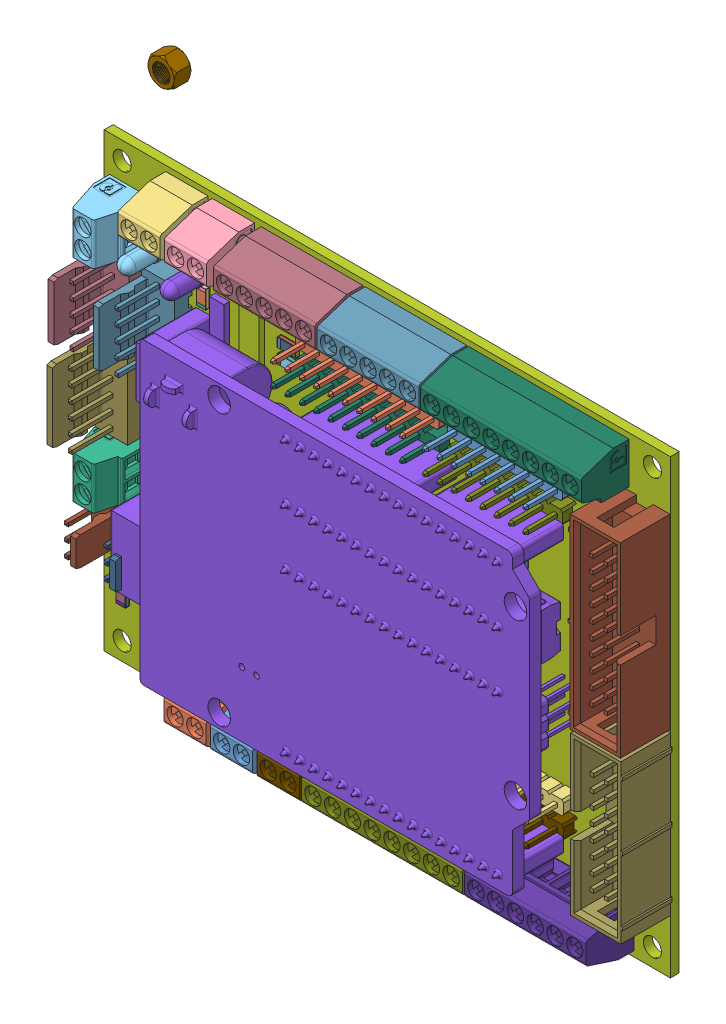
SolidWorks assembly Arduino Uno shield with Unokk, configuration Standard. Lengths in mm.
Overall size (100.65 90.35 23.92).
193 component instances, 191 part files, 2 mates.
Components (placement in the parent):
- PPP5f08ec48b7509.stp-1: PPP5f08ec48b7509.stp [Standard] at origin size (100.65 80.01 15.26)
  - CAPRR500W50L750T250H650P002.stp-1: CAPRR500W50L750T250H650P002.stp [Standard] at (21.59 34.29 1.57) x (0 -1 0) z (0 0 1) size (7.5 2.5 6.5)
  - CAPRR500W50L750T250H650P001.stp-1: CAPRR500W50L750T250H650P001.stp [Standard] at (21.59 34.29 1.57) x (0 -1 0) z (0 0 1) size (0.5 0.5 6.5)
  - CAPRR500W50L750T250H650P.stp-1: CAPRR500W50L750T250H650P.stp [Standard] at (21.59 34.29 1.57) x (0 -1 0) z (0 0 1) size (0.5 0.5 6.5)
  - CAPRR500W50L750T250H650P003.stp-1: CAPRR500W50L750T250H650P003.stp [Standard] at (20.32 26.67 1.57) x (0 -1 0) z (0 0 1) size (7.5 2.5 6.5)
  - CAPRR500W50L750T250H650P004.stp-1: CAPRR500W50L750T250H650P004.stp [Standard] at (20.32 26.67 1.57) x (0 -1 0) z (0 0 1) size (0.5 0.5 6.5)
  - CAPRR500W50L750T250H650P005.stp-1: CAPRR500W50L750T250H650P005.stp [Standard] at (20.32 26.67 1.57) x (0 -1 0) z (0 0 1) size (0.5 0.5 6.5)
  - Component_1.stp-1: Component_1.stp [Standard] at (26.67 60.325 1.57) x (0 1 0) z (0 0 1) size (15.24 3.56 1)
  - SW3dPS-MELF_Cylinder5.stp-1: SW3dPS-MELF_Cylinder5.stp [Standard] at (33.02 13.208 1.57) x (0 1 0) z (0 0 1) size (0.5 2.5 2.5)
  - SW3dPS-MELF_Cylinder7.stp-1: SW3dPS-MELF_Cylinder7.stp [Standard] at (33.02 13.208 1.57) x (0 1 0) z (0 0 1) size (0.8 2.5 2.5)
  - SW3dPS-MELF_Board1.stp-1: SW3dPS-MELF_Board1.stp [Standard] at (33.02 13.208 1.57) x (0 1 0) z (0 0 1) size (1.7 0.01 0.01)
  - SW3dPS-MELF_Cylinder9.stp-1: SW3dPS-MELF_Cylinder9.stp [Standard] at (33.02 13.208 1.57) x (0 1 0) z (0 0 1) size (2.4 2.5 2.5)
  - SW3dPS-MELF_Cylinder8.stp-1: SW3dPS-MELF_Cylinder8.stp [Standard] at (33.02 13.208 1.57) x (0 1 0) z (0 0 1) size (0.5 2.5 2.5)
  - SW3dPS-MELF_Cylinder6.stp-1: SW3dPS-MELF_Cylinder6.stp [Standard] at (33.02 13.208 1.57) x (0 1 0) z (0 0 1) size (0.8 2.5 2.5)
  - SW3dPS-MELF_Cylinder010.stp-1: SW3dPS-MELF_Cylinder010.stp [Standard] at (41.275 13.208 1.57) x (0 1 0) z (0 0 1) size (0.5 2.5 2.5)
  - SW3dPS-MELF_Cylinder011.stp-1: SW3dPS-MELF_Cylinder011.stp [Standard] at (41.275 13.208 1.57) x (0 1 0) z (0 0 1) size (0.8 2.5 2.5)
  - SW3dPS-MELF_Board002.stp-1: SW3dPS-MELF_Board002.stp [Standard] at (41.275 13.208 1.57) x (0 1 0) z (0 0 1) size (1.7 0.01 0.01)
  - SW3dPS-MELF_Cylinder012.stp-1: SW3dPS-MELF_Cylinder012.stp [Standard] at (41.275 13.208 1.57) x (0 1 0) z (0 0 1) size (2.4 2.5 2.5)
  - SW3dPS-MELF_Cylinder013.stp-1: SW3dPS-MELF_Cylinder013.stp [Standard] at (41.275 13.208 1.57) x (0 1 0) z (0 0 1) size (0.5 2.5 2.5)
  - SW3dPS-MELF_Cylinder014.stp-1: SW3dPS-MELF_Cylinder014.stp [Standard] at (41.275 13.208 1.57) x (0 1 0) z (0 0 1) size (0.8 2.5 2.5)
  - SW3dPS-MELF_Cylinder015.stp-1: SW3dPS-MELF_Cylinder015.stp [Standard] at (24.765 13.208 1.57) x (0 1 0) z (0 0 1) size (0.5 2.5 2.5)
  - SW3dPS-MELF_Cylinder016.stp-1: SW3dPS-MELF_Cylinder016.stp [Standard] at (24.765 13.208 1.57) x (0 1 0) z (0 0 1) size (0.8 2.5 2.5)
  - SW3dPS-MELF_Board003.stp-1: SW3dPS-MELF_Board003.stp [Standard] at (24.765 13.208 1.57) x (0 1 0) z (0 0 1) size (1.7 0.01 0.01)
  - SW3dPS-MELF_Cylinder017.stp-1: SW3dPS-MELF_Cylinder017.stp [Standard] at (24.765 13.208 1.57) x (0 1 0) z (0 0 1) size (2.4 2.5 2.5)
  - SW3dPS-MELF_Cylinder018.stp-1: SW3dPS-MELF_Cylinder018.stp [Standard] at (24.765 13.208 1.57) x (0 1 0) z (0 0 1) size (0.5 2.5 2.5)
  - SW3dPS-MELF_Cylinder019.stp-1: SW3dPS-MELF_Cylinder019.stp [Standard] at (24.765 13.208 1.57) x (0 1 0) z (0 0 1) size (0.8 2.5 2.5)
  - Component_2.stp-1: Component_2.stp [Standard] at (20.955 59.69 1.57) x (0 -1 0) z (0 0 1) size (10.16 2.54 1)
  - Component_3.stp-1: Component_3.stp [Standard] at (20.32 43.815 1.57) x (-1 0 0) z (0 0 1) size (10.16 3.17 1)
  - =_[0_1_1_2].stp-1: =_[0_1_1_2].stp [Standard] at (10.795 24.13 1.57) x (0 -1 0) z (0 0 1) size (7.62 5.8 15.26)
  - =_[0_1_1_2]001.stp-1: =_[0_1_1_2]001.stp [Standard] at (3.81 24.13 1.57) x (0 -1 0) z (0 0 1) size (7.62 5.8 15.26)
  - =_[0_1_1_2]002.stp-1: =_[0_1_1_2]002.stp [Standard] at (4.445 44.45 1.57) x (0 1 0) z (0 0 1) size (15.24 5.8 15.26)
  - =_[0_1_1_2]003.stp-1: =_[0_1_1_2]003.stp [Standard] at (4.699 59.055 1.57) x (0 1 0) z (0 0 1) size (12.7 5.8 15.26)
  - =_[0_1_1_2]004.stp-1: =_[0_1_1_2]004.stp [Standard] at (12.7 59.055 1.57) x (0 1 0) z (0 0 1) size (12.7 5.8 15.26)
  - 1.stp-1: 1.stp [Standard] at (49.276 63.5 1.57) x (-1 0 0) z (0 0 1) size (25.4 2.5 11.2)
  - 1001.stp-1: 1001.stp [Standard] at (73.66 63.5 1.57) x (-1 0 0) z (0 0 1) size (20.32 2.5 11.2)
  - 1002.stp-1: 1002.stp [Standard] at (55.88 15.24 1.57) x (-1 0 0) z (0 0 1) size (20.32 2.5 11.2)
  - 1003.stp-1: 1003.stp [Standard] at (76.2 15.24 1.57) size (15.24 2.5 11.2)
  - 1004.stp-1: 1004.stp [Standard] at (73.66 67.31 1.57) x (-1 0 0) z (0 0 1) size (20.32 2.5 11.2)
  - 1005.stp-1: 1005.stp [Standard] at (49.276 67.31 1.57) x (-1 0 0) z (0 0 1) size (25.4 2.5 11.2)
  - 1006.stp-1: 1006.stp [Standard] at (76.2 19.05 1.57) size (15.24 2.5 11.2)
  - 1007.stp-1: 1007.stp [Standard] at (55.88 19.05 1.57) x (-1 0 0) z (0 0 1) size (20.32 2.5 11.2)
  - LEDRD254W000D310H620P002.stp-1: LEDRD254W000D310H620P002.stp [Standard] at (12.065 69.215 1.57) x (0 1 0) z (0 0 1) size (3.1 3.1 6.2)
  - LEDRD254W000D310H620P.stp-1: LEDRD254W000D310H620P.stp [Standard] at (12.065 69.215 1.57) x (0 1 0) z (0 0 1) size (0.38 0.38 6.2)
  - LEDRD254W000D310H620P001.stp-1: LEDRD254W000D310H620P001.stp [Standard] at (12.065 69.215 1.57) x (0 1 0) z (0 0 1) size (0.38 0.38 6.2)
  - LEDRD254W000D310H620P003.stp-1: LEDRD254W000D310H620P003.stp [Standard] at (19.685 69.215 1.57) x (0 1 0) z (0 0 1) size (3.1 3.1 6.2)
  - LEDRD254W000D310H620P004.stp-1: LEDRD254W000D310H620P004.stp [Standard] at (19.685 69.215 1.57) x (0 1 0) z (0 0 1) size (0.38 0.38 6.2)
  - LEDRD254W000D310H620P005.stp-1: LEDRD254W000D310H620P005.stp [Standard] at (19.685 69.215 1.57) x (0 1 0) z (0 0 1) size (0.38 0.38 6.2)
  - LEDRD254W000D310H620P006.stp-1: LEDRD254W000D310H620P006.stp [Standard] at (50.8 52.705 1.57) x (-1 0 0) z (0 0 1) size (3.1 3.1 6.2)
  - LEDRD254W000D310H620P007.stp-1: LEDRD254W000D310H620P007.stp [Standard] at (50.8 52.705 1.57) x (-1 0 0) z (0 0 1) size (0.38 0.38 6.2)
  - LEDRD254W000D310H620P008.stp-1: LEDRD254W000D310H620P008.stp [Standard] at (50.8 52.705 1.57) x (-1 0 0) z (0 0 1) size (0.38 0.38 6.2)
  - LEDRD254W000D310H620P009.stp-1: LEDRD254W000D310H620P009.stp [Standard] at (45.72 52.705 1.57) x (-1 0 0) z (0 0 1) size (3.1 3.1 6.2)
  - LEDRD254W000D310H620P010.stp-1: LEDRD254W000D310H620P010.stp [Standard] at (45.72 52.705 1.57) x (-1 0 0) z (0 0 1) size (0.38 0.38 6.2)
  - LEDRD254W000D310H620P011.stp-1: LEDRD254W000D310H620P011.stp [Standard] at (45.72 52.705 1.57) x (-1 0 0) z (0 0 1) size (0.38 0.38 6.2)
  - User_Library-TO263-3New_Extruded_2.stp-1: User_Library-TO263-3New_Extruded_2.stp [Standard] at (41.91 31.75 1.57) x (-1 0 0) z (0 0 1) size (1.4 1.53 0.51)
  - User_Library-TO263-3New_Extruded.stp-1: User_Library-TO263-3New_Extruded.stp [Standard] at (41.91 31.75 1.57) x (-1 0 0) z (0 0 1) size (1 5.77 3.36)
  - User_Library-TO263-3New_D2PACK.stp-1: User_Library-TO263-3New_D2PACK.stp [Standard] at (41.91 31.75 1.57) x (-1 0 0) z (0 0 1) size (10.41 15.85 4.61)
  - User_Library-TO263-3New_Extruded_003.stp-1: User_Library-TO263-3New_Extruded_003.stp [Standard] at (54.61 31.75 1.57) x (-1 0 0) z (0 0 1) size (1.4 1.53 0.51)
  - User_Library-TO263-3New_Extruded001.stp-1: User_Library-TO263-3New_Extruded001.stp [Standard] at (54.61 31.75 1.57) x (-1 0 0) z (0 0 1) size (1 5.77 3.36)
  - User_Library-TO263-3New_D2PACK001.stp-1: User_Library-TO263-3New_D2PACK001.stp [Standard] at (54.61 31.75 1.57) x (-1 0 0) z (0 0 1) size (10.41 15.85 4.61)
  - User_Library-TO263-3New_Extruded_004.stp-1: User_Library-TO263-3New_Extruded_004.stp [Standard] at (29.21 31.75 1.57) x (-1 0 0) z (0 0 1) size (1.4 1.53 0.51)
  - User_Library-TO263-3New_Extruded002.stp-1: User_Library-TO263-3New_Extruded002.stp [Standard] at (29.21 31.75 1.57) x (-1 0 0) z (0 0 1) size (1 5.77 3.36)
  - User_Library-TO263-3New_D2PACK002.stp-1: User_Library-TO263-3New_D2PACK002.stp [Standard] at (29.21 31.75 1.57) x (-1 0 0) z (0 0 1) size (10.41 15.85 4.61)
  - RESC3216X078.stp-1: RESC3216X078.stp [Standard] at (54.483 46.482 1.57) size (2.12 1.6 0.1)
  - RESC3216X079.stp-1: RESC3216X079.stp [Standard] at (54.483 46.482 1.57) size (3.06 1.6 0.56)
  - RESC3216X077.stp-1: RESC3216X077.stp [Standard] at (54.483 46.482 1.57) size (0.57 1.6 0.76)
  - RESC3216X080.stp-1: RESC3216X080.stp [Standard] at (54.483 46.482 1.57) size (2.12 1.6 0.1)
  - RESC3216X76.stp-1: RESC3216X76.stp [Standard] at (54.483 46.482 1.57) size (0.57 1.6 0.76)
  - RESC3216X081.stp-1: RESC3216X081.stp [Standard] at (41.91 46.355 1.57) size (2.12 1.6 0.1)
  - RESC3216X082.stp-1: RESC3216X082.stp [Standard] at (41.91 46.355 1.57) size (3.06 1.6 0.56)
  - RESC3216X083.stp-1: RESC3216X083.stp [Standard] at (41.91 46.355 1.57) size (0.57 1.6 0.76)
  - RESC3216X084.stp-1: RESC3216X084.stp [Standard] at (41.91 46.355 1.57) size (2.12 1.6 0.1)
  - RESC3216X085.stp-1: RESC3216X085.stp [Standard] at (41.91 46.355 1.57) size (0.57 1.6 0.76)
  - RESC3216X086.stp-1: RESC3216X086.stp [Standard] at (29.21 48.895 1.57) size (2.12 1.6 0.1)
  - RESC3216X087.stp-1: RESC3216X087.stp [Standard] at (29.21 48.895 1.57) size (3.06 1.6 0.56)
  - RESC3216X088.stp-1: RESC3216X088.stp [Standard] at (29.21 48.895 1.57) size (0.57 1.6 0.76)
  - RESC3216X089.stp-1: RESC3216X089.stp [Standard] at (29.21 48.895 1.57) size (2.12 1.6 0.1)
  - RESC3216X090.stp-1: RESC3216X090.stp [Standard] at (29.21 48.895 1.57) size (0.57 1.6 0.76)
  - RESC3216X091.stp-1: RESC3216X091.stp [Standard] at (33.02 60.96 1.57) size (2.12 1.6 0.1)
  - RESC3216X092.stp-1: RESC3216X092.stp [Standard] at (33.02 60.96 1.57) size (3.06 1.6 0.56)
  - RESC3216X093.stp-1: RESC3216X093.stp [Standard] at (33.02 60.96 1.57) size (0.57 1.6 0.76)
  - RESC3216X094.stp-1: RESC3216X094.stp [Standard] at (33.02 60.96 1.57) size (2.12 1.6 0.1)
  - RESC3216X095.stp-1: RESC3216X095.stp [Standard] at (33.02 60.96 1.57) size (0.57 1.6 0.76)
  - RESC3216X096.stp-1: RESC3216X096.stp [Standard] at (33.02 63.5 1.57) size (2.12 1.6 0.1)
  - RESC3216X097.stp-1: RESC3216X097.stp [Standard] at (33.02 63.5 1.57) size (3.06 1.6 0.56)
  - RESC3216X098.stp-1: RESC3216X098.stp [Standard] at (33.02 63.5 1.57) size (0.57 1.6 0.76)
  - RESC3216X099.stp-1: RESC3216X099.stp [Standard] at (33.02 63.5 1.57) size (2.12 1.6 0.1)
  - RESC3216X100.stp-1: RESC3216X100.stp [Standard] at (33.02 63.5 1.57) size (0.57 1.6 0.76)
  - RESC3216X101.stp-1: RESC3216X101.stp [Standard] at (15.875 69.215 1.57) x (0 -1 0) z (0 0 1) size (2.12 1.6 0.1)
  - RESC3216X102.stp-1: RESC3216X102.stp [Standard] at (15.875 69.215 1.57) x (0 -1 0) z (0 0 1) size (3.06 1.6 0.56)
  - RESC3216X103.stp-1: RESC3216X103.stp [Standard] at (15.875 69.215 1.57) x (0 -1 0) z (0 0 1) size (0.57 1.6 0.76)
  - RESC3216X104.stp-1: RESC3216X104.stp [Standard] at (15.875 69.215 1.57) x (0 -1 0) z (0 0 1) size (2.12 1.6 0.1)
  - RESC3216X105.stp-1: RESC3216X105.stp [Standard] at (15.875 69.215 1.57) x (0 -1 0) z (0 0 1) size (0.57 1.6 0.76)
  - RESC3216X106.stp-1: RESC3216X106.stp [Standard] at (17.907 63.627 1.57) x (0 1 0) z (0 0 1) size (2.12 1.6 0.1)
  - RESC3216X107.stp-1: RESC3216X107.stp [Standard] at (17.907 63.627 1.57) x (0 1 0) z (0 0 1) size (3.06 1.6 0.56)
  - RESC3216X108.stp-1: RESC3216X108.stp [Standard] at (17.907 63.627 1.57) x (0 1 0) z (0 0 1) size (0.57 1.6 0.76)
  - RESC3216X109.stp-1: RESC3216X109.stp [Standard] at (17.907 63.627 1.57) x (0 1 0) z (0 0 1) size (2.12 1.6 0.1)
  - RESC3216X110.stp-1: RESC3216X110.stp [Standard] at (17.907 63.627 1.57) x (0 1 0) z (0 0 1) size (0.57 1.6 0.76)
  - RESC3216X111.stp-1: RESC3216X111.stp [Standard] at (50.673 57.023 1.57) x (-1 0 0) z (0 0 1) size (2.12 1.6 0.1)
  - RESC3216X112.stp-1: RESC3216X112.stp [Standard] at (50.673 57.023 1.57) x (-1 0 0) z (0 0 1) size (3.06 1.6 0.56)
  - RESC3216X113.stp-1: RESC3216X113.stp [Standard] at (50.673 57.023 1.57) x (-1 0 0) z (0 0 1) size (0.57 1.6 0.76)
  - RESC3216X114.stp-1: RESC3216X114.stp [Standard] at (50.673 57.023 1.57) x (-1 0 0) z (0 0 1) size (2.12 1.6 0.1)
  - RESC3216X115.stp-1: RESC3216X115.stp [Standard] at (50.673 57.023 1.57) x (-1 0 0) z (0 0 1) size (0.57 1.6 0.76)
  - RESC3216X116.stp-1: RESC3216X116.stp [Standard] at (46.99 57.277 1.57) x (0 -1 0) z (0 0 1) size (2.12 1.6 0.1)
  - RESC3216X117.stp-1: RESC3216X117.stp [Standard] at (46.99 57.277 1.57) x (0 -1 0) z (0 0 1) size (3.06 1.6 0.56)
  - RESC3216X118.stp-1: RESC3216X118.stp [Standard] at (46.99 57.277 1.57) x (0 -1 0) z (0 0 1) size (0.57 1.6 0.76)
  - RESC3216X119.stp-1: RESC3216X119.stp [Standard] at (46.99 57.277 1.57) x (0 -1 0) z (0 0 1) size (2.12 1.6 0.1)
  - RESC3216X120.stp-1: RESC3216X120.stp [Standard] at (46.99 57.277 1.57) x (0 -1 0) z (0 0 1) size (0.57 1.6 0.76)
  - RESC3216X121.stp-1: RESC3216X121.stp [Standard] at (34.925 45.085 1.57) x (-1 0 0) z (0 0 1) size (2.12 1.6 0.1)
  - RESC3216X122.stp-1: RESC3216X122.stp [Standard] at (34.925 45.085 1.57) x (-1 0 0) z (0 0 1) size (3.06 1.6 0.56)
  - RESC3216X123.stp-1: RESC3216X123.stp [Standard] at (34.925 45.085 1.57) x (-1 0 0) z (0 0 1) size (0.57 1.6 0.76)
  - RESC3216X124.stp-1: RESC3216X124.stp [Standard] at (34.925 45.085 1.57) x (-1 0 0) z (0 0 1) size (2.12 1.6 0.1)
  - RESC3216X125.stp-1: RESC3216X125.stp [Standard] at (34.925 45.085 1.57) x (-1 0 0) z (0 0 1) size (0.57 1.6 0.76)
  - RESC3216X126.stp-1: RESC3216X126.stp [Standard] at (47.625 46.101 1.57) x (0 -1 0) z (0 0 1) size (2.12 1.6 0.1)
  - RESC3216X127.stp-1: RESC3216X127.stp [Standard] at (47.625 46.101 1.57) x (0 -1 0) z (0 0 1) size (3.06 1.6 0.56)
  - RESC3216X128.stp-1: RESC3216X128.stp [Standard] at (47.625 46.101 1.57) x (0 -1 0) z (0 0 1) size (0.57 1.6 0.76)
  - RESC3216X129.stp-1: RESC3216X129.stp [Standard] at (47.625 46.101 1.57) x (0 -1 0) z (0 0 1) size (2.12 1.6 0.1)
  - RESC3216X130.stp-1: RESC3216X130.stp [Standard] at (47.625 46.101 1.57) x (0 -1 0) z (0 0 1) size (0.57 1.6 0.76)
  - RESC3216X131.stp-1: RESC3216X131.stp [Standard] at (59.69 48.006 1.57) x (0 -1 0) z (0 0 1) size (2.12 1.6 0.1)
  - RESC3216X132.stp-1: RESC3216X132.stp [Standard] at (59.69 48.006 1.57) x (0 -1 0) z (0 0 1) size (3.06 1.6 0.56)
  - RESC3216X133.stp-1: RESC3216X133.stp [Standard] at (59.69 48.006 1.57) x (0 -1 0) z (0 0 1) size (0.57 1.6 0.76)
  - RESC3216X134.stp-1: RESC3216X134.stp [Standard] at (59.69 48.006 1.57) x (0 -1 0) z (0 0 1) size (2.12 1.6 0.1)
  - RESC3216X135.stp-1: RESC3216X135.stp [Standard] at (59.69 48.006 1.57) x (0 -1 0) z (0 0 1) size (0.57 1.6 0.76)
  - RESC2012X072.stp-1: RESC2012X072.stp [Standard] at (10.795 50.165 1.57) x (-1 0 0) z (0 0 1) size (1.2 1.25 0.1)
  - RESC2012X073.stp-1: RESC2012X073.stp [Standard] at (10.795 50.165 1.57) x (-1 0 0) z (0 0 1) size (1.8 1.25 0.5)
  - RESC2012X071.stp-1: RESC2012X071.stp [Standard] at (10.795 50.165 1.57) x (-1 0 0) z (0 0 1) size (0.4 1.25 0.7)
  - RESC2012X074.stp-1: RESC2012X074.stp [Standard] at (10.795 50.165 1.57) x (-1 0 0) z (0 0 1) size (1.2 1.25 0.1)
  - RESC2012X70.stp-1: RESC2012X70.stp [Standard] at (10.795 50.165 1.57) x (-1 0 0) z (0 0 1) size (0.4 1.25 0.7)
  - RESC2012X075.stp-1: RESC2012X075.stp [Standard] at (10.795 47.625 1.57) x (-1 0 0) z (0 0 1) size (1.2 1.25 0.1)
  - RESC2012X076.stp-1: RESC2012X076.stp [Standard] at (10.795 47.625 1.57) x (-1 0 0) z (0 0 1) size (1.8 1.25 0.5)
  - RESC2012X077.stp-1: RESC2012X077.stp [Standard] at (10.795 47.625 1.57) x (-1 0 0) z (0 0 1) size (0.4 1.25 0.7)
  - RESC2012X078.stp-1: RESC2012X078.stp [Standard] at (10.795 47.625 1.57) x (-1 0 0) z (0 0 1) size (1.2 1.25 0.1)
  - RESC2012X079.stp-1: RESC2012X079.stp [Standard] at (10.795 47.625 1.57) x (-1 0 0) z (0 0 1) size (0.4 1.25 0.7)
  - RESC2012X080.stp-1: RESC2012X080.stp [Standard] at (10.795 45.085 1.57) x (-1 0 0) z (0 0 1) size (1.2 1.25 0.1)
  - RESC2012X081.stp-1: RESC2012X081.stp [Standard] at (10.795 45.085 1.57) x (-1 0 0) z (0 0 1) size (1.8 1.25 0.5)
  - RESC2012X082.stp-1: RESC2012X082.stp [Standard] at (10.795 45.085 1.57) x (-1 0 0) z (0 0 1) size (0.4 1.25 0.7)
  - RESC2012X083.stp-1: RESC2012X083.stp [Standard] at (10.795 45.085 1.57) x (-1 0 0) z (0 0 1) size (1.2 1.25 0.1)
  - RESC2012X084.stp-1: RESC2012X084.stp [Standard] at (10.795 45.085 1.57) x (-1 0 0) z (0 0 1) size (0.4 1.25 0.7)
  - RESC2012X085.stp-1: RESC2012X085.stp [Standard] at (10.795 42.545 1.57) x (-1 0 0) z (0 0 1) size (1.2 1.25 0.1)
  - RESC2012X086.stp-1: RESC2012X086.stp [Standard] at (10.795 42.545 1.57) x (-1 0 0) z (0 0 1) size (1.8 1.25 0.5)
  - RESC2012X087.stp-1: RESC2012X087.stp [Standard] at (10.795 42.545 1.57) x (-1 0 0) z (0 0 1) size (0.4 1.25 0.7)
  - RESC2012X088.stp-1: RESC2012X088.stp [Standard] at (10.795 42.545 1.57) x (-1 0 0) z (0 0 1) size (1.2 1.25 0.1)
  - RESC2012X089.stp-1: RESC2012X089.stp [Standard] at (10.795 42.545 1.57) x (-1 0 0) z (0 0 1) size (0.4 1.25 0.7)
  - RESC2012X090.stp-1: RESC2012X090.stp [Standard] at (10.795 40.005 1.57) x (-1 0 0) z (0 0 1) size (1.2 1.25 0.1)
  - RESC2012X091.stp-1: RESC2012X091.stp [Standard] at (10.795 40.005 1.57) x (-1 0 0) z (0 0 1) size (1.8 1.25 0.5)
  - RESC2012X092.stp-1: RESC2012X092.stp [Standard] at (10.795 40.005 1.57) x (-1 0 0) z (0 0 1) size (0.4 1.25 0.7)
  - RESC2012X093.stp-1: RESC2012X093.stp [Standard] at (10.795 40.005 1.57) x (-1 0 0) z (0 0 1) size (1.2 1.25 0.1)
  - RESC2012X094.stp-1: RESC2012X094.stp [Standard] at (10.795 40.005 1.57) x (-1 0 0) z (0 0 1) size (0.4 1.25 0.7)
  - RESC2012X095.stp-1: RESC2012X095.stp [Standard] at (10.795 37.465 1.57) x (-1 0 0) z (0 0 1) size (1.2 1.25 0.1)
  - RESC2012X096.stp-1: RESC2012X096.stp [Standard] at (10.795 37.465 1.57) x (-1 0 0) z (0 0 1) size (1.8 1.25 0.5)
  - RESC2012X097.stp-1: RESC2012X097.stp [Standard] at (10.795 37.465 1.57) x (-1 0 0) z (0 0 1) size (0.4 1.25 0.7)
  - RESC2012X098.stp-1: RESC2012X098.stp [Standard] at (10.795 37.465 1.57) x (-1 0 0) z (0 0 1) size (1.2 1.25 0.1)
  - RESC2012X099.stp-1: RESC2012X099.stp [Standard] at (10.795 37.465 1.57) x (-1 0 0) z (0 0 1) size (0.4 1.25 0.7)
  - RESC3216X136.stp-1: RESC3216X136.stp [Standard] at (64.135 32.639 1.57) x (0 1 0) z (0 0 1) size (2.12 1.6 0.1)
  - RESC3216X137.stp-1: RESC3216X137.stp [Standard] at (64.135 32.639 1.57) x (0 1 0) z (0 0 1) size (3.06 1.6 0.56)
  - RESC3216X138.stp-1: RESC3216X138.stp [Standard] at (64.135 32.639 1.57) x (0 1 0) z (0 0 1) size (0.57 1.6 0.76)
  - RESC3216X139.stp-1: RESC3216X139.stp [Standard] at (64.135 32.639 1.57) x (0 1 0) z (0 0 1) size (2.12 1.6 0.1)
  - RESC3216X140.stp-1: RESC3216X140.stp [Standard] at (64.135 32.639 1.57) x (0 1 0) z (0 0 1) size (0.57 1.6 0.76)
  - RESC3216X141.stp-1: RESC3216X141.stp [Standard] at (3.683 10.795 1.57) x (0 1 0) z (0 0 1) size (2.12 1.6 0.1)
  - RESC3216X142.stp-1: RESC3216X142.stp [Standard] at (3.683 10.795 1.57) x (0 1 0) z (0 0 1) size (3.06 1.6 0.56)
  - RESC3216X143.stp-1: RESC3216X143.stp [Standard] at (3.683 10.795 1.57) x (0 1 0) z (0 0 1) size (0.57 1.6 0.76)
  - RESC3216X144.stp-1: RESC3216X144.stp [Standard] at (3.683 10.795 1.57) x (0 1 0) z (0 0 1) size (2.12 1.6 0.1)
  - RESC3216X145.stp-1: RESC3216X145.stp [Standard] at (3.683 10.795 1.57) x (0 1 0) z (0 0 1) size (0.57 1.6 0.76)
  - RESC3216X146.stp-1: RESC3216X146.stp [Standard] at (74.422 51.943 1.57) x (0 -1 0) z (0 0 1) size (2.12 1.6 0.1)
  - RESC3216X147.stp-1: RESC3216X147.stp [Standard] at (74.422 51.943 1.57) x (0 -1 0) z (0 0 1) size (3.06 1.6 0.56)
  - RESC3216X148.stp-1: RESC3216X148.stp [Standard] at (74.422 51.943 1.57) x (0 -1 0) z (0 0 1) size (0.57 1.6 0.76)
  - RESC3216X149.stp-1: RESC3216X149.stp [Standard] at (74.422 51.943 1.57) x (0 -1 0) z (0 0 1) size (2.12 1.6 0.1)
  - RESC3216X150.stp-1: RESC3216X150.stp [Standard] at (74.422 51.943 1.57) x (0 -1 0) z (0 0 1) size (0.57 1.6 0.76)
  - RESC3216X151.stp-1: RESC3216X151.stp [Standard] at (3.683 17.272 1.57) x (0 1 0) z (0 0 1) size (2.12 1.6 0.1)
  - RESC3216X152.stp-1: RESC3216X152.stp [Standard] at (3.683 17.272 1.57) x (0 1 0) z (0 0 1) size (3.06 1.6 0.56)
  - RESC3216X153.stp-1: RESC3216X153.stp [Standard] at (3.683 17.272 1.57) x (0 1 0) z (0 0 1) size (0.57 1.6 0.76)
  - RESC3216X154.stp-1: RESC3216X154.stp [Standard] at (3.683 17.272 1.57) x (0 1 0) z (0 0 1) size (2.12 1.6 0.1)
  - RESC3216X155.stp-1: RESC3216X155.stp [Standard] at (3.683 17.272 1.57) x (0 1 0) z (0 0 1) size (0.57 1.6 0.76)
  - Component_4.stp-1: Component_4.stp [Standard] at (11.684 10.287 1.57) size (2 2 1)
  - User_Library-BH-10...64.stp-1: User_Library-BH-10...64.stp [Standard] at (95.885 54.61 1.57) x (0 1 0) z (0 0 1) size (33.06 9.2 12.14)
  - User_Library-BH-10...065.stp-1: User_Library-BH-10...065.stp [Standard] at (95.885 23.495 1.57) x (0 -1 0) z (0 0 1) size (27.98 9.2 12.14)
  - mkds_1-5-3.5_mkds_1-5-3.5;mkds_1-5-3.5.stp-1: mkds_1-5-3.5_mkds_1-5-3.5;mkds_1-5-3.5.stp [Standard] at (36.83 75.565 1.57) size (18 7.3 12)
  - mkds_1-5-3.5_mkds_1-5-3.5;mkds_1-5-3.006.stp-1: mkds_1-5-3.5_mkds_1-5-3.5;mkds_1-5-3.006.stp [Standard] at (55.245 75.565 1.57) size (18 7.3 12)
  - mkds_1-8-3.5_mkds_1-8-3.5;mkds_1-8-3.5.stp-1: mkds_1-8-3.5_mkds_1-8-3.5;mkds_1-8-3.5.stp [Standard] at (78.74 75.565 1.57) size (28.5 7.3 12)
  - mkds_1-8-3.5_mkds_1-8-3.5;mkds_1-8-3.006.stp-1: mkds_1-8-3.5_mkds_1-8-3.5;mkds_1-8-3.006.stp [Standard] at (57.785 4.445 1.57) x (-1 0 0) z (0 0 1) size (28.5 7.3 12)
  - mkds_1-6-3.5_mkds_1-6-3.5;mkds_1-6-3.5.stp-1: mkds_1-6-3.5_mkds_1-6-3.5;mkds_1-6-3.5.stp [Standard] at (83.185 4.445 1.57) x (-1 0 0) z (0 0 1) size (21.5 7.3 12)
  - mkds_1-2-3.5_mkds_1-2-3.5;mkds_1-2-3.5.stp-1: mkds_1-2-3.5_mkds_1-2-3.5;mkds_1-2-3.5.stp [Standard] at (39.37 4.445 1.57) x (-1 0 0) z (0 0 1) size (7.5 7.3 12)
  - mkds_1-2-3.5_mkds_1-2-3.5;mkds_1-2-3.006.stp-1: mkds_1-2-3.5_mkds_1-2-3.5;mkds_1-2-3.006.stp [Standard] at (31.115 4.445 1.57) x (-1 0 0) z (0 0 1) size (7.5 7.3 12)
  - mkds_1-2-3.5_mkds_1-2-3.5;mkds_1-2-3.007.stp-1: mkds_1-2-3.5_mkds_1-2-3.5;mkds_1-2-3.007.stp [Standard] at (22.86 4.445 1.57) x (-1 0 0) z (0 0 1) size (7.5 7.3 12)
  - mkds_1-2-3.5_mkds_1-2-3.5;mkds_1-2-3.008.stp-1: mkds_1-2-3.5_mkds_1-2-3.5;mkds_1-2-3.008.stp [Standard] at (14.605 75.565 1.57) size (7.5 7.3 12)
  - mkds_1-2-3.5_mkds_1-2-3.5;mkds_1-2-3.009.stp-1: mkds_1-2-3.5_mkds_1-2-3.5;mkds_1-2-3.009.stp [Standard] at (22.86 75.565 1.57) size (7.5 7.3 12)
  - mkds_1-2-3.5_mkds_1-2-3.5;mkds_1-2-3.010.stp-1: mkds_1-2-3.5_mkds_1-2-3.5;mkds_1-2-3.010.stp [Standard] at (4.445 69.85 1.57) x (0 1 0) z (0 0 1) size (7.5 7.3 12)
  - mkds_1-2-3.5_mkds_1-2-3.5;mkds_1-2-3.011.stp-1: mkds_1-2-3.5_mkds_1-2-3.5;mkds_1-2-3.011.stp [Standard] at (4.445 32.385 1.57) x (0 1 0) z (0 0 1) size (7.5 7.3 12)
  - Component_Component.stp-1: Component_Component.stp [Standard] at origin size (100.33 80.01 1.57)
- arduino uno-2: arduino uno [Default] at (52.02 37.3929 14.21) x (1 0 0) z (0 1 0) size (76.5 14.6 53)
- kkkkk-2: kkkkk [Default] at (132.8181 -85.8824 -60.2258) x (0.934285 0.356528 0) z (0 0 1) size (6.55 6.85 3.19)
  - Part3^kkkkk-1: Part3^kkkkk [Default] at origin (virtual)
  - Part2^kkkkk-1: Part2^kkkkk [Default] at origin (virtual)
  - nut (1) (1)-1: nut (1) (1) [Default] at (-59.1167 207.857 53.7136) x (0.966766 -0.255664 0) z (0 0 1) size (5.28 5.69 3.19)
Mates (geometry in assembly coordinates):
- Deckungsgleich2: coincident anti-aligned: plane of PPP5f08ec48b7509.stp-1/1006.stp-1 through (69.95 19.0531 4.11) normal (0 0 1); plane of arduino uno-2 through (52.02 37.3929 4.11) normal (0 0 -1)
- Deckungsgleich3: coincident aligned: line of PPP5f08ec48b7509.stp-1/1006.stp-1 through (83.92 19.9013 4.11) axis (0 -1 0); line of arduino uno-2 through (83.92 14.2929 4.11) axis (0 -1 0)
